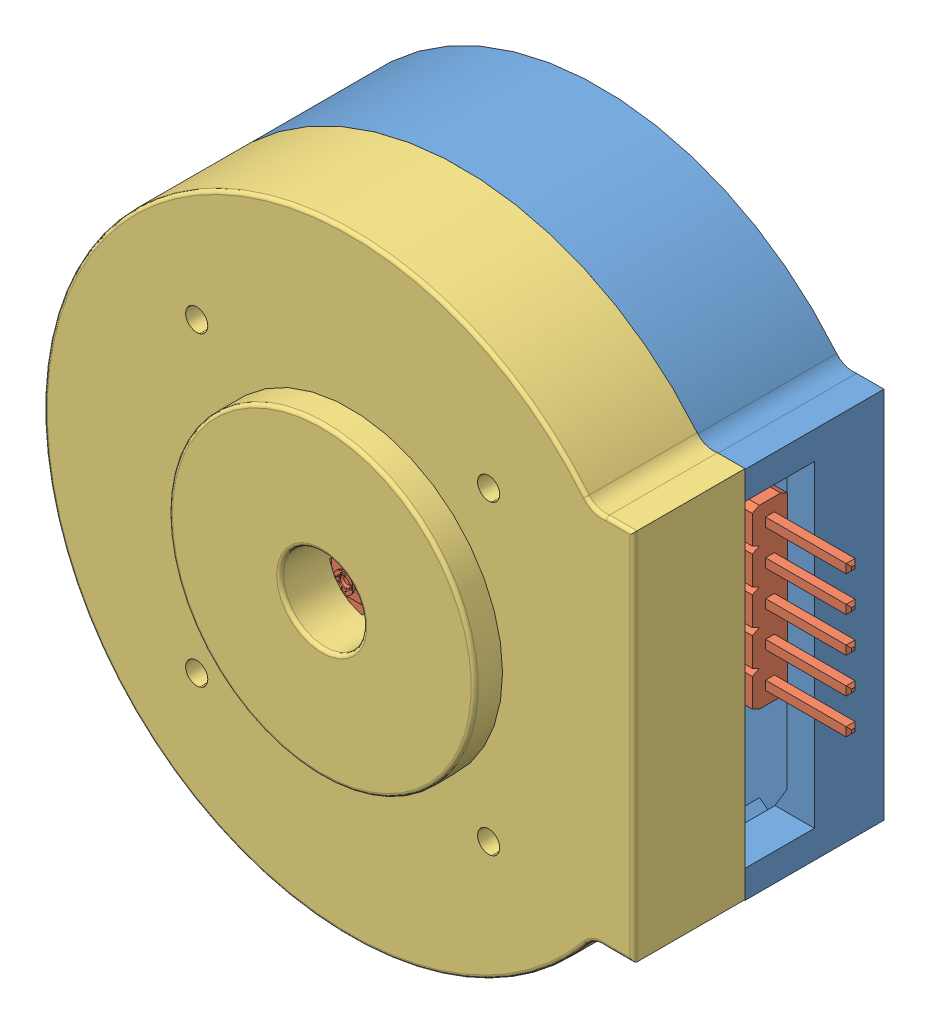
SolidWorks assembly Assem2, configuration Default. Lengths in mm.
Overall size (48.55 44 20).
3 component instances, 3 part files, 6 mates.
Components (placement in the parent):
- base_sensor-1: base_sensor [Default] at (4.5408 -34.6336 21.1827) size (42.43 44 10)
- final-sensor.step-1: final-sensor.step [Default] at (4.5383 -34.636 31.1842) size (47.26 41.3 8.75)
- cap_sensor-1: cap_sensor [Default] at (4.5408 -34.6336 39.1827) x (1 0 0) z (0 0 -1) size (42.43 44 10)
Mates (geometry in assembly coordinates):
- Coincident10: coincident anti-aligned: plane of base_sensor-1 through (4.5408 -34.6336 31.1827) normal (0 0 1); plane of cap_sensor-1 through (4.5408 -34.6336 31.1827) normal (0 0 -1)
- Concentric3: concentric anti-aligned: cylinder of base_sensor-1 through (4.5408 -34.6336 31.1827) axis (0 0 -1) radius 22; cylinder of cap_sensor-1 through (4.5408 -34.6336 31.1827) axis (0 0 1) radius 22
- Coincident11: coincident aligned: plane of base_sensor-1 through (24.9745 -20.3057 21.1817) normal (1 0 0); plane of cap_sensor-1 through (24.9745 -48.9616 39.1837) normal (1 0 0)
- Coincident18: coincident anti-aligned: plane of base_sensor-1 through (4.5408 -34.6336 30.7727) normal (0 0 1); plane of final-sensor.step-1 through (-16.1667 -37.098 30.7727) normal (0 0 -1)
- Parallel9: parallel aligned: plane of base_sensor-1 through (24.9745 -20.3057 21.1817) normal (1 0 0); plane of final-sensor.step-1 through (22.9523 -23.836 30.7727) normal (1 0 0)
- Concentric20: concentric anti-aligned: cylinder of base_sensor-1 through (4.5408 -34.6336 12.6827) axis (0 0 1) radius 3; cylinder of final-sensor.step-1 through (4.5408 -34.6336 30.7727) axis (0 0 -1) radius 2.5025
